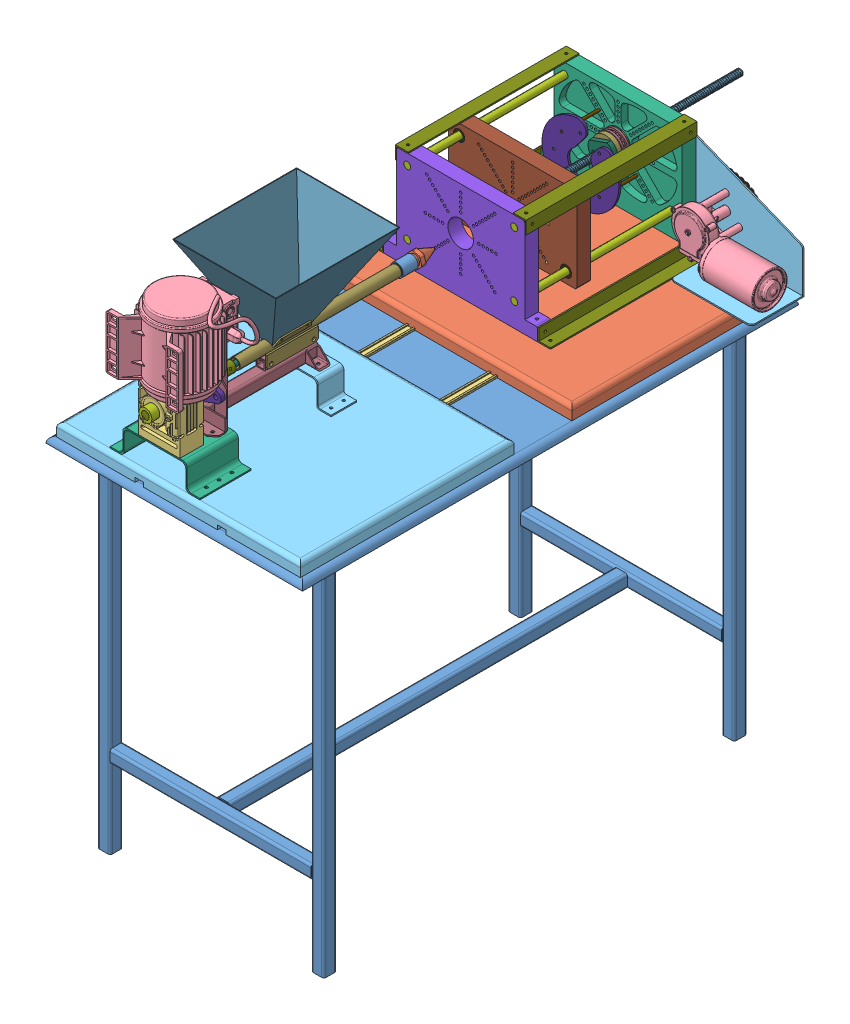
SolidWorks assembly Collection, configuration Default. Lengths in mm.
Overall size (638.2 1318.78 1465.86).
145 component instances, 46 part files, 26 mates.
Components (placement in the parent):
- table-1: table [Default<As Machined>] at (913.5416 -7.4669 1379.7888) size (600 860 1160)
- table inj-1: table inj [Default] at (601.6185 277.6613 334.7888) x (0 0 -1) z (0 1 0) size (500 570 30)
- Slid one-1: Slid one [Default] at (805.208 277.6613 834.7888) size (20 5 300)
- Slidtow-1: Slidtow [Default] at (803.208 278.6613 969.9122) size (20 10 300)
- Slidtow-2: Slidtow [Default] at (995.7971 278.6613 969.9122) size (20 10 300)
- Slid one-2: Slid one [Default] at (997.7971 277.6613 834.7888) size (20 5 300)
- tablw Ex-1: tablw Ex [Default] at (1171.6185 277.6613 1469.9122) x (0 0 1) z (0 1 0) size (500 570 30)
- newAssmblyy-1: newAssmblyy [Default] at (461.6185 447.1783 353.0211) x (1 0 0) z (0 0 -1) size (613.2 233 659.47)
  - fram 1-1: fram 1 [Default] at (360 9.5169 -23.7677) size (360 230 32)
  - Rod-1: Rod [Default] at (235 -65.4831 -391.7677) x (0.626545 0.779385 0) z (0 0 1) size (16 16 400)
  - Rod-2: Rod [Default] at (485 -65.4831 -391.7677) x (0.626545 0.779385 0) z (0 0 1) size (16 16 400)
  - Rod-3: Rod [Default] at (235 84.5169 -391.7677) x (-0.446951 0.894559 0) z (0 0 1) size (16 16 400)
  - Rod-4: Rod [Default] at (485 84.5169 -391.7677) x (0.626545 0.779385 0) z (0 0 1) size (16 16 400)
  - fram 2-1: fram 2 [Default] at (360 9.5169 -359.7677) x (-1 0 0) z (0 0 -1) size (360 230 32)
  - Fram3Bearing-1: Fram3Bearing [Default] at (239.4857 -63.2792 -253.8232) x (0 0 1) z (-0.755658 -0.654967 0) size (18.32 26.4 26.4)
    - needle roller bearing_nh_iso-1: needle roller bearing_nh_iso [ISO 3245 - 1622D - 14,DE,AC,14] at (-10.7976 1.2726 4.8331) size (12 24 24)
    - cag-1: cag [Default] at (-16.4776 1.2726 4.8331) x (0 0.015498 -0.99988) z (1 0 0) size (26 26 18)
  - fram 3-1: fram 3 [Default] at (360 9.5169 -238.3008) x (-1 0 0) z (0 0 -1) size (300 200 32)
  - Fram3Bearing-5: Fram3Bearing [Default] at (489.9953 -65.6427 -253.8232) x (0 0 1) z (-0.974675 -0.223625 0) size (18.32 26.4 26.4)
    - needle roller bearing_nh_iso-1: needle roller bearing_nh_iso [ISO 3245 - 1622D - 14,DE,AC,14] at (-10.7976 1.2726 4.8331) size (12 24 24)
    - cag-1: cag [Default] at (-16.4776 1.2726 4.8331) x (0 0.015498 -0.99988) z (1 0 0) size (26 26 18)
  - Fram3Bearing-6: Fram3Bearing [Default] at (239.9486 83.817 -253.8232) x (0 0 1) z (-0.993167 -0.116703 0) size (18.32 26.4 26.4)
    - needle roller bearing_nh_iso-1: needle roller bearing_nh_iso [ISO 3245 - 1622D - 14,DE,AC,14] at (-10.7976 1.2726 4.8331) size (12 24 24)
    - cag-1: cag [Default] at (-16.4776 1.2726 4.8331) x (0 0.015498 -0.99988) z (1 0 0) size (26 26 18)
  - Fram3Bearing-7: Fram3Bearing [Default] at (489.9979 84.5114 -253.8232) x (0 0 1) z (-0.96732 -0.253559 0) size (18.32 26.4 26.4)
    - needle roller bearing_nh_iso-1: needle roller bearing_nh_iso [ISO 3245 - 1622D - 14,DE,AC,14] at (-10.7976 1.2726 4.8331) size (12 24 24)
    - cag-1: cag [Default] at (-16.4776 1.2726 4.8331) x (0 0.015498 -0.99988) z (1 0 0) size (26 26 18)
  - Bearing fram 1-1: Bearing fram 1 [Default] at (359.6336 10.028 -20.0582) x (0 0 1) z (-0.908257 -0.418414 0) size (14 62 62)
    - angular contact ball bearing_68_iso-1: angular contact ball bearing_68_iso [ISO 15 ABB - 1035 - Full,DE,AC,Full_68] at (1.2904 -0.6174 -0.1189) size (14 62 62) (hidden)
  - Bearing fram 1-2: Bearing fram 1 [Default] at (360.0098 8.8882 -20.0582) x (0 0 1) z (0.984776 -0.173828 0) size (14 62 62)
    - angular contact ball bearing_68_iso-1: angular contact ball bearing_68_iso [ISO 15 ABB - 1035 - Full,DE,AC,Full_68] at (1.2904 -0.6174 -0.1189) size (14 62 62) (hidden)
  - scrowHome-2: scrowHome [Default] at (360 9.5169 -43.7677) x (-0.746779 -0.665072 0) z (0 0 -1) size (60 60 120.41)
  - LoadBearing fram 1-3: LoadBearing fram 1 [Default] at (354.2089 2.6537 0.389) x (0 0 -1) z (0.633402 0.773823 0) size (18 62 62)
    - thrust ball bearing_68_iso-1: thrust ball bearing_68_iso [ISO 104 - 123562 - B,12,DE,NC,12_68] at (-16.8432 -0.1341 8.9791) size (18 62 62)
  - LoadBearing fram 1-5: LoadBearing fram 1 [Default] at (351.0209 9.651 -51.611) x (0 0 -1) z (1 0 0) size (18 62 62)
    - thrust ball bearing_68_iso-1: thrust ball bearing_68_iso [ISO 104 - 123562 - B,12,DE,NC,12_68] at (-16.8432 -0.1341 8.9791) size (18 62 62)
  - bollScrow (1)-1: bollScrow (1) [Default] at (360 9.5169 -238.3008) x (0.848557 0.529104 0) z (0 0 1) size (15.39 15.68 509.99)
  - bollSrcewhome-1: bollSrcewhome [Default] at (360 9.5169 -28.7677) x (0.940959 -0.338519 0) z (0 0 1) size (60 40 39.69)
  - SideFram-1: SideFram [Default] at (237 -90.4831 8.2323) x (1 0 0) z (0 0 -1) size (30 30 400)
  - SideFram-2: SideFram [Default] at (570 136.5169 -391.7677) size (30 30 400)
  - SideFram-3: SideFram [Default] at (510 -63.4831 8.2323) x (0 1 0) z (0 0 -1) size (30 30 400)
  - SideFram-4: SideFram [Default] at (150 136.5169 8.2323) x (-1 0 0) z (0 0 -1) size (30 30 400)
  - Ring -1: Ring  [Default] at (360 9.5169 -111.7677) size (180 179.69 5)
  - Rod Of The Ring -1: Rod Of The Ring  [Default] at (404.1942 53.7111 -111.7677) x (0.195075 0.980788 0) z (0 0 1) size (6 6 120)
  - Rod Of The Ring -2: Rod Of The Ring  [Default] at (315.8058 -34.6772 -111.7677) size (6 6 120)
  - Cuopling-1: Cuopling [Default] at (360 9.5169 -223.3008) x (-0.849668 -0.527317 0) z (0 0 1) size (30 30 55.36)
  - rod slid-1: rod slid [Default] at (292.0495 26.0952 -214.3008) x (-1 0 0) z (0 0 1) size (200 120 4)
  - Rod Of The Rod Slid-1: Rod Of The Rod Slid [Default] at (442.5 9.5169 -270.3008) x (0.999971 -0.007577 0) z (0 0 1) size (6 6 60)
  - Rod Of The Rod Slid-2: Rod Of The Rod Slid [Default] at (439.5495 89.0664 -270.3008) x (0.998743 0.050114 0) z (0 0 1) size (6 6 60)
  - Rod Of The Rod Slid-4: Rod Of The Rod Slid [Default] at (277.5 9.5169 -270.3008) size (6 6 60)
  - Rod Of The Rod Slid-5: Rod Of The Rod Slid [Default] at (280.4505 89.0664 -270.3008) size (6 6 60)
  - Wiper_motor_1-1: Wiper_motor_1 [Varsayılan] at (652.4379 95.5169 -58.7677) x (0 1 0) z (0 0 1) size (128 227.07 138.6)
  - motor case-1: motor case [Default] at (570 136.5169 8.2323) x (1 0 0) z (0 0 -1) size (300 218.23 123)
  - LockGear-1: LockGear [Default] at (360 9.5169 30.2323) x (0.274686 -0.961534 0) z (0 0 1) size (60 60 23.07) (hidden)
  - spring2-1: spring2 [Default] at (442.5 9.5169 -215.4008) size (11.73 12.66 23.3)
  - spring2-2: spring2 [Default] at (439.5495 89.0664 -215.4008) size (11.73 12.66 23.3)
  - spring2-3: spring2 [Default] at (280.4505 89.0664 -215.4008) size (11.73 12.66 23.3)
  - spring2-4: spring2 [Default] at (277.5 9.5169 -215.4008) size (11.73 12.66 23.3)
  - Chainsprocket-1: Chainsprocket [Default] at (535.0439 -10.9424 28.2323) x (-0.98179 -0.189971 0) z (0 0 1) size (345.21 131.8 15.57)
    - Path-1: Path [Default] at origin
    - Sprocket-2: Sprocket [Default] at (167.9697 -53.34 -2) x (-0.998781 -0.049354 0) z (0 0 1) size (113.38 112.55 4.69)
    - Innerchain-1: Innerchain [Default] at (220.2759 -45.0398 -7.2786) x (-0.156725 0.987642 0) z (0 0 1) size (23.62 10.92 15.57)
    - Outerchain-1: Outerchain [Default] at (216.803 -32.8603 5.5499) x (-0.386746 0.922186 0) z (0 0 -1) size (25 12.19 11.1)
    - Innerchain-2: Innerchain [Default] at (210.5494 -21.8471 -7.2786) x (-0.594647 0.803987 0) z (0 0 1) size (23.62 10.92 15.57)
    - Innerchain-3: Innerchain [Default] at (191.2209 -5.7562 -7.2786) x (-0.898474 0.439027 0) z (0 0 1) size (23.62 10.92 15.57)
    - Innerchain-4: Innerchain [Default] at (166.6482 -0.1187 -7.2786) x (-0.999825 0.018697 0) z (0 0 1) size (23.62 10.92 15.57)
    - Innerchain-5: Innerchain [Default] at (141.1365 0 -7.2786) x (-1 0 0) z (0 0 1) size (23.62 10.92 15.57)
    - Innerchain-6: Innerchain [Default] at (115.6236 0 -7.2786) x (-1 0 0) z (0 0 1) size (23.62 10.92 15.57)
    - Innerchain-7: Innerchain [Default] at (90.1108 0 -7.2786) x (-1 0 0) z (0 0 1) size (23.62 10.92 15.57)
    - Innerchain-8: Innerchain [Default] at (64.5979 0 -7.2786) x (-1 0 0) z (0 0 1) size (23.62 10.92 15.57)
    - Innerchain-9: Innerchain [Default] at (39.0851 0 -7.2786) x (-1 0 0) z (0 0 1) size (23.62 10.92 15.57)
    - Innerchain-10: Innerchain [Default] at (13.5722 0 -7.2786) x (-1 0 0) z (0 0 1) size (23.62 10.92 15.57)
    - Innerchain-11: Innerchain [Default] at (-11.9406 0 -7.2786) x (-1 0 0) z (0 0 1) size (23.62 10.92 15.57)
    - Innerchain-12: Innerchain [Default] at (-37.4535 0 -7.2786) x (-1 0 0) z (0 0 1) size (23.62 10.92 15.57)
    - Innerchain-13: Innerchain [Default] at (-62.9304 -0.674 -7.2786) x (-0.99435 -0.106149 0) z (0 0 1) size (23.62 10.92 15.57)
    - Innerchain-14: Innerchain [Default] at (-86.592 -9.1985 -7.2786) x (-0.833477 -0.552554 0) z (0 0 1) size (23.62 10.92 15.57)
    - Innerchain-15: Innerchain [Default] at (-103.6546 -27.6747 -7.2786) x (-0.48461 -0.87473 0) z (0 0 1) size (23.62 10.92 15.57)
    - Innerchain-16: Innerchain [Default] at (-110.2705 -51.9386 -7.2786) x (-0.026461 -0.99965 0) z (0 0 1) size (23.62 10.92 15.57)
    - Innerchain-17: Innerchain [Default] at (-104.9475 -76.5185 -7.2786) x (0.437656 -0.899143 0) z (0 0 1) size (23.62 10.92 15.57)
    - Innerchain-18: Innerchain [Default] at (-88.8862 -95.8716 -7.2786) x (0.803078 -0.595874 0) z (0 0 1) size (23.62 10.92 15.57)
    - Innerchain-19: Innerchain [Default] at (-65.7746 -105.9835 -7.2786) x (0.976975 -0.213356 0) z (0 0 1) size (23.62 10.92 15.57)
    - Innerchain-20: Innerchain [Default] at (-40.7106 -110.7247 -7.2786) x (0.986708 -0.162503 0) z (0 0 1) size (23.62 10.92 15.57)
    - Innerchain-21: Innerchain [Default] at (-15.4561 -114.3259 -7.2786) x (0.992802 -0.119768 0) z (0 0 1) size (23.62 10.92 15.57)
    - Innerchain-22: Innerchain [Default] at (9.9302 -116.8339 -7.2786) x (0.997046 -0.07681 0) z (0 0 1) size (23.62 10.92 15.57)
    - Innerchain-23: Innerchain [Default] at (35.4011 -118.2438 -7.2786) x (0.999432 -0.033708 0) z (0 0 1) size (23.62 10.92 15.57)
    - Innerchain-24: Innerchain [Default] at (60.9091 -118.5532 -7.2786) x (0.999955 0.009457 0) z (0 0 1) size (23.62 10.92 15.57)
    - Innerchain-25: Innerchain [Default] at (86.4067 -117.7615 -7.2786) x (0.998615 0.052604 0) z (0 0 1) size (23.62 10.92 15.57)
    - Innerchain-26: Innerchain [Default] at (111.8464 -115.87 -7.2786) x (0.995415 0.095652 0) z (0 0 1) size (23.62 10.92 15.57)
    - Innerchain-27: Innerchain [Default] at (137.1807 -112.8824 -7.2786) x (0.990359 0.138523 0) z (0 0 1) size (23.62 10.92 15.57)
    - Innerchain-28: Innerchain [Default] at (162.3625 -108.8043 -7.2786) x (0.983458 0.181136 0) z (0 0 1) size (23.62 10.92 15.57)
    - Innerchain-29: Innerchain [Default] at (187.0706 -102.7362 -7.2786) x (0.932696 0.360663 0) z (0 0 1) size (23.62 10.92 15.57)
    - Innerchain-30: Innerchain [Default] at (207.7031 -88.3555 -7.2786) x (0.66116 0.750245 0) z (0 0 1) size (23.62 10.92 15.57)
    - Innerchain-31: Innerchain [Default] at (219.3755 -66.0786 -7.2786) x (0.240529 0.970642 0) z (0 0 1) size (23.62 10.92 15.57)
    - Outerchain-2: Outerchain [Default] at (201.8498 -12.6429 5.5499) x (-0.768539 0.639803 0) z (0 0 -1) size (25 12.19 11.1)
    - Outerchain-3: Outerchain [Default] at (179.2563 -1.6029 5.5499) x (-0.977021 0.213141 0) z (0 0 -1) size (25 12.19 11.1)
    - Outerchain-4: Outerchain [Default] at (153.8929 0 5.5499) x (-1 0 0) z (0 0 -1) size (25 12.19 11.1)
    - Outerchain-5: Outerchain [Default] at (128.3801 0 5.5499) x (-1 0 0) z (0 0 -1) size (25 12.19 11.1)
    - Outerchain-6: Outerchain [Default] at (102.8672 0 5.5499) x (-1 0 0) z (0 0 -1) size (25 12.19 11.1)
    - Outerchain-7: Outerchain [Default] at (77.3544 0 5.5499) x (-1 0 0) z (0 0 -1) size (25 12.19 11.1)
    - Outerchain-8: Outerchain [Default] at (51.8415 0 5.5499) x (-1 0 0) z (0 0 -1) size (25 12.19 11.1)
    - Outerchain-9: Outerchain [Default] at (26.3287 0 5.5499) x (-1 0 0) z (0 0 -1) size (25 12.19 11.1)
    - Outerchain-10: Outerchain [Default] at (0.8158 0 5.5499) x (-1 0 0) z (0 0 -1) size (25 12.19 11.1)
    - Outerchain-11: Outerchain [Default] at (-24.697 0 5.5499) x (-1 0 0) z (0 0 -1) size (25 12.19 11.1)
    - Outerchain-12: Outerchain [Default] at (-50.2099 0 5.5499) x (-1 0 0) z (0 0 -1) size (25 12.19 11.1)
    - Outerchain-13: Outerchain [Default] at (-75.272 -3.5189 5.5499) x (-0.940839 -0.338854 0) z (0 0 -1) size (25 12.19 11.1)
    - Outerchain-14: Outerchain [Default] at (-96.231 -17.4137 5.5499) x (-0.678445 -0.734651 0) z (0 0 -1) size (25 12.19 11.1)
    - Outerchain-15: Outerchain [Default] at (-108.4172 -39.4101 5.5499) x (-0.263058 -0.96478 0) z (0 0 -1) size (25 12.19 11.1)
    - Outerchain-16: Outerchain [Default] at (-109.0826 -64.5477 5.5499) x (0.21165 -0.977345 0) z (0 0 -1) size (25 12.19 11.1)
    - Outerchain-17: Outerchain [Default] at (-98.0771 -87.1579 5.5499) x (0.63863 -0.769514 0) z (0 0 -1) size (25 12.19 11.1)
    - Outerchain-18: Outerchain [Default] at (-77.8825 -102.142 5.5499) x (0.921595 -0.388153 0) z (0 0 -1) size (25 12.19 11.1)
    - Outerchain-19: Outerchain [Default] at (-53.2735 -108.5156 5.5499) x (0.982971 -0.183763 0) z (0 0 -1) size (25 12.19 11.1)
    - Outerchain-20: Outerchain [Default] at (-28.1027 -112.661 5.5499) x (0.989986 -0.141169 0) z (0 0 -1) size (25 12.19 11.1)
    - Outerchain-21: Outerchain [Default] at (-2.7764 -115.7163 5.5499) x (0.995156 -0.098312 0) z (0 0 -1) size (25 12.19 11.1)
    - Outerchain-22: Outerchain [Default] at (22.6581 -117.6757 5.5499) x (0.998471 -0.055272 0) z (0 0 -1) size (25 12.19 11.1)
    - Outerchain-23: Outerchain [Default] at (48.1534 -118.5356 5.5499) x (0.999926 -0.012128 0) z (0 0 -1) size (25 12.19 11.1)
    - Outerchain-24: Outerchain [Default] at (73.6622 -118.2943 5.5499) x (0.999518 0.031037 0) z (0 0 -1) size (25 12.19 11.1)
    - Outerchain-25: Outerchain [Default] at (99.1367 -116.9524 5.5499) x (0.997247 0.074145 0) z (0 0 -1) size (25 12.19 11.1)
    - Outerchain-26: Outerchain [Default] at (124.5296 -114.5123 5.5499) x (0.993118 0.117115 0) z (0 0 -1) size (25 12.19 11.1)
    - Outerchain-27: Outerchain [Default] at (149.7935 -110.9786 5.5499) x (0.987139 0.159867 0) z (0 0 -1) size (25 12.19 11.1)
    - Outerchain-28: Outerchain [Default] at (174.8777 -106.3402 5.5499) x (0.978746 0.205077 0) z (0 0 -1) size (25 12.19 11.1)
    - Outerchain-29: Outerchain [Default] at (198.249 -96.7828 5.5499) x (0.820389 0.571806 0) z (0 0 -1) size (25 12.19 11.1)
    - Outerchain-30: Outerchain [Default] at (214.8748 -77.9168 5.5499) x (0.464117 0.885774 0) z (0 0 -1) size (25 12.19 11.1)
    - Outerchain-31: Outerchain [Default] at (220.9233 -53.5086 5.5499) x (0.003184 0.999995 0) z (0 0 -1) size (25 12.19 11.1)
    - Sprocket 2-1: Sprocket 2 [Default] at (-57.3283 -53.34 0) x (0.999995 -0.003296 0) z (0 0 1) size (113.38 112.55 4.69)
  - LockGear-2: LockGear [Default] at (360 9.5169 30.2323) x (-0.124758 0.992187 0) z (0 0 1) size (60 60 23.07)
- Extrusion -1: Extrusion  [Default] at (1919.1794 239.0342 27.9211) x (0.073366 0.997163 0.016854) z (0.091086 -0.023528 0.995565) size (418.43 284.89 726.82)
  - Part1^Extrusion -1: Part1^Extrusion  [Default] at origin (virtual)
  - extrusion barrel-1: extrusion barrel [Default] at (129.5902 1170.4061 607.1747) x (0.997163 0.071506 -0.023528) z (-0.016854 -0.092553 -0.995565) size (57.45 48.09 390.48)
  - extrusion barrel holder-1: extrusion barrel holder [Default<As Machined>] at (80.5853 1198.8633 956.9179) x (-0.073366 0.993137 -0.091086) z (-0.016854 -0.092553 -0.995565) size (120 103 290)
  - extrusion hopper-1: extrusion hopper [Default] at (134.0526 1194.9302 870.9997) x (-0.997163 -0.071506 0.023528) z (0.016854 0.092553 0.995565) size (200 241.59 290)
  - Screwnew-1: Screwnew [Default] at (138.7635 1220.7812 1149.0421) x (-0.763007 0.644678 -0.047016) z (-0.016854 -0.092553 -0.995565) size (22.44 22.43 457.9)
  - extrusion barrel shaft-1: extrusion barrel shaft [Default] at (140.7543 1231.7135 1266.637) x (-0.016854 -0.092553 -0.995565) z (-0.884682 0.465336 -0.028284) size (200 25 25)
  - LoadBearing -1: LoadBearing  [Default] at (143.3106 1231.7289 1209.5223) x (0.016854 0.092553 0.995565) z (-0.995565 -0.090616 0.025278) size (10 35 35)
    - thrust ball bearing_68_iso-1: thrust ball bearing_68_iso [ISO 104 - 112035 - B,14,DE,AC,14_68] at (-1.1831 -4.9542 3.9901) size (10 35 35)
  - bearing Home-1: bearing Home [Default] at (361.7918 1143.6724 1228.491) x (0.069598 -0.9934 0.091174) z (-0.016854 -0.092553 -0.995565) size (115 52.7 15)
  - Bearing -1: Bearing  [Default] at (131.894 1229.4198 1233.7636) x (0.016854 0.092553 0.995565) z (0.948116 -0.317638 0.013479) size (14 42 42)
    - angular contact ball bearing_68_iso-4: angular contact ball bearing_68_iso [ISO 15 ABB - 2020 - Full,DE,NC,Full_68] at (-12.9108 -1.9168 8.1151) size (14 42 42)
  - Muff-1: Muff [Default] at (131.5498 1181.167 722.926) x (-0.603313 0.794957 -0.06369) z (0.016854 0.092553 0.995565) size (30 30 35.96)
  - nozzel Extrouder-1: nozzel Extrouder [Default] at (130.6936 1176.4652 672.3509) x (0.649958 -0.757643 0.059432) z (0.016854 0.092553 0.995565) size (35.05 33.8 65.48)
  - GearBox-1: GearBox [Default] at (141.8995 1224.7406 1293.9843) x (-0.016854 -0.092553 -0.995565) z (-0.997163 -0.071506 0.023528) size (90 116 125.24)
  - Motor-1: Motor [默认] at (286.3938 1212.6382 1292.6633) x (-0.073366 0.993137 -0.091086) z (-0.997163 -0.071506 0.023528) size (207.5 187.3 268.32)
  - extrusion barrel holder 2 Base -1: extrusion barrel holder 2 Base  [Default] at (69.781 1136.7744 947.8505) x (0.073391 -0.993 0.092551) z (0.016746 0.094015 0.99543) size (180.8 59.94 60)
  - extrusion barrel holder 1 Base-1: extrusion barrel holder 1 Base [Default] at (64.2883 1295.1367 1196.3439) x (-0.073366 0.993137 -0.091086) z (-0.016854 -0.092553 -0.995565) size (210 59.94 120)
  - gearboxCuopling-1: gearboxCuopling [Default] at (133.5287 1237.5846 1288.3115) x (0.46589 0.880282 -0.089723) z (0.016854 0.092553 0.995565) size (30 30 55)
  - key-1: key [Default] at (134.2226 1242.9583 1343.0452) x (-0.46589 -0.880282 0.089723) z (-0.016854 -0.092553 -0.995565) size (4 4.7 50)
Mates (geometry in assembly coordinates):
- Coincident4: coincident anti-aligned: plane of table-1 through (913.5416 277.6613 1379.7888) normal (0 1 0); plane of Slid one-1 through (805.208 277.6613 1134.7888) normal (0 -1 0)
- Coincident7: coincident anti-aligned: plane of table-1 through (913.5416 277.6613 1379.7888) normal (0 1 0); plane of table inj-1 through (601.6185 277.6613 334.7888) normal (0 -1 0)
- Coincident8: coincident aligned: line of table-1 through (1171.6185 277.6613 334.7888) axis (-1 0 0); line of table inj-1 through (1171.6185 277.6613 334.7888) axis (-1 0 0)
- Coincident9: coincident aligned: line of table-1 through (601.6185 277.6613 334.7888) axis (0 0 1); line of table inj-1 through (601.6185 277.6613 334.7888) axis (0 0 1)
- Coincident10: coincident anti-aligned: plane of table inj-1 through (601.6185 307.6613 834.7888) normal (0 0 1); plane of Slid one-1 through (805.208 277.6613 834.7888) normal (0 0 -1)
- Coincident11: coincident anti-aligned: plane of Slid one-1 through (805.208 278.6613 1134.7888) normal (0 1 0); plane of Slidtow-1 through (803.208 278.6613 1269.9122) normal (0 -1 0)
- Coincident12: coincident anti-aligned: plane of Slid one-1 through (787.208 277.6613 1134.7888) normal (1 0 0); plane of Slidtow-1 through (787.208 278.6613 1269.9122) normal (-1 0 0)
- Coincident13: coincident anti-aligned: plane of Slidtow-2 through (995.7971 278.6613 1269.9122) normal (0 -1 0); plane of Slid one-2 through (997.7971 278.6613 1134.7888) normal (0 1 0)
- Coincident14: coincident anti-aligned: plane of Slidtow-2 through (979.7971 278.6613 1269.9122) normal (-1 0 0); plane of Slid one-2 through (979.7971 277.6613 1134.7888) normal (1 0 0)
- Coincident15: coincident anti-aligned: plane of table inj-1 through (601.6185 307.6613 834.7888) normal (0 0 1); plane of Slid one-2 through (997.7971 277.6613 834.7888) normal (0 0 -1)
- Coincident16: coincident anti-aligned: plane of table-1 through (913.5416 277.6613 1379.7888) normal (0 1 0); plane of Slid one-2 through (997.7971 277.6613 1134.7888) normal (0 -1 0)
- LimitDistance1: limit distance = 135.1234 mm aligned: plane of Slidtow-2 through (995.7971 278.6613 969.9122) normal (0 0 -1); plane of Slid one-2 through (997.7971 277.6613 834.7888) normal (0 0 -1)
- LimitDistance2: limit distance = 135.1234 mm aligned: plane of Slidtow-1 through (803.208 278.6613 969.9122) normal (0 0 -1); plane of Slid one-1 through (805.208 277.6613 834.7888) normal (0 0 -1)
- Coincident18: coincident anti-aligned: plane of table-1 through (913.5416 277.6613 1379.7888) normal (0 1 0); plane of tablw Ex-1 through (1171.6185 277.6613 1469.9122) normal (0 -1 0)
- Coincident33: coincident anti-aligned: plane of Slid one-2 through (997.7971 277.6613 1134.7888) normal (1 0 0); plane of tablw Ex-1 through (997.7971 287.6613 1469.9122) normal (-1 0 0)
- Coincident34: coincident anti-aligned: plane of Slid one-1 through (785.208 277.6613 1134.7888) normal (-1 0 0); plane of tablw Ex-1 through (785.208 287.6613 1469.9122) normal (1 0 0)
- Coincident35: coincident aligned: plane of Slidtow-1 through (803.208 278.6613 969.9122) normal (0 0 -1); plane of tablw Ex-1 through (1171.6185 307.6613 969.9122) normal (0 0 -1)
- Coincident36: coincident aligned: plane of Slidtow-2 through (995.7971 278.6613 969.9122) normal (0 0 -1); plane of tablw Ex-1 through (1171.6185 307.6613 969.9122) normal (0 0 -1)
- Coincident37: coincident aligned: line of table-1 through (601.6185 277.6613 334.7888) axis (0 0 1); line of tablw Ex-1 through (601.6185 277.6613 969.9122) axis (0 0 1)
- Coincident38: coincident anti-aligned: plane of table inj-1 through (601.6185 307.6613 334.7888) normal (0 1 0); plane of newAssmblyy-1/fram 1-1 through (1001.6185 307.6613 344.7888) normal (0 -1 0)
- Coincident39: coincident anti-aligned: line of table inj-1 through (1161.6185 307.6613 344.7888) axis (-1 0 0); line of newAssmblyy-1/fram 1-1 through (641.6185 307.6613 344.7888) axis (1 0 0)
- Coincident41: coincident anti-aligned: line of table inj-1 through (611.6185 307.6613 344.7888) axis (0 0 1); line of newAssmblyy-1/SideFram-4 through (611.6185 307.6613 744.7888) axis (0 0 -1)
- Coincident42: coincident anti-aligned: plane of tablw Ex-1 through (1171.6185 307.6613 1469.9122) normal (0 1 0); plane of Extrusion -1/extrusion barrel holder 2 Base -1 through (760.7739 307.6613 1137.7786) normal (0 -1 0)
- Concentric1: concentric aligned: cylinder of newAssmblyy-1/fram 2-1 through (821.6185 437.6613 744.7888) axis (0 0 -1) radius 30; cylinder of Extrusion -1/Muff-1 through (821.6185 437.6613 894.1792) axis (0 0 -1) radius 15
- Coincident43: coincident aligned: line of tablw Ex-1 through (611.6185 307.6613 1459.9122) axis (1 0 0); line of Extrusion -1/extrusion barrel holder 1 Base-1 through (716.6179 307.6613 1459.9122) axis (1 0 0)
- Lock1: lock: unknown of tablw Ex-1; unknown of ?
